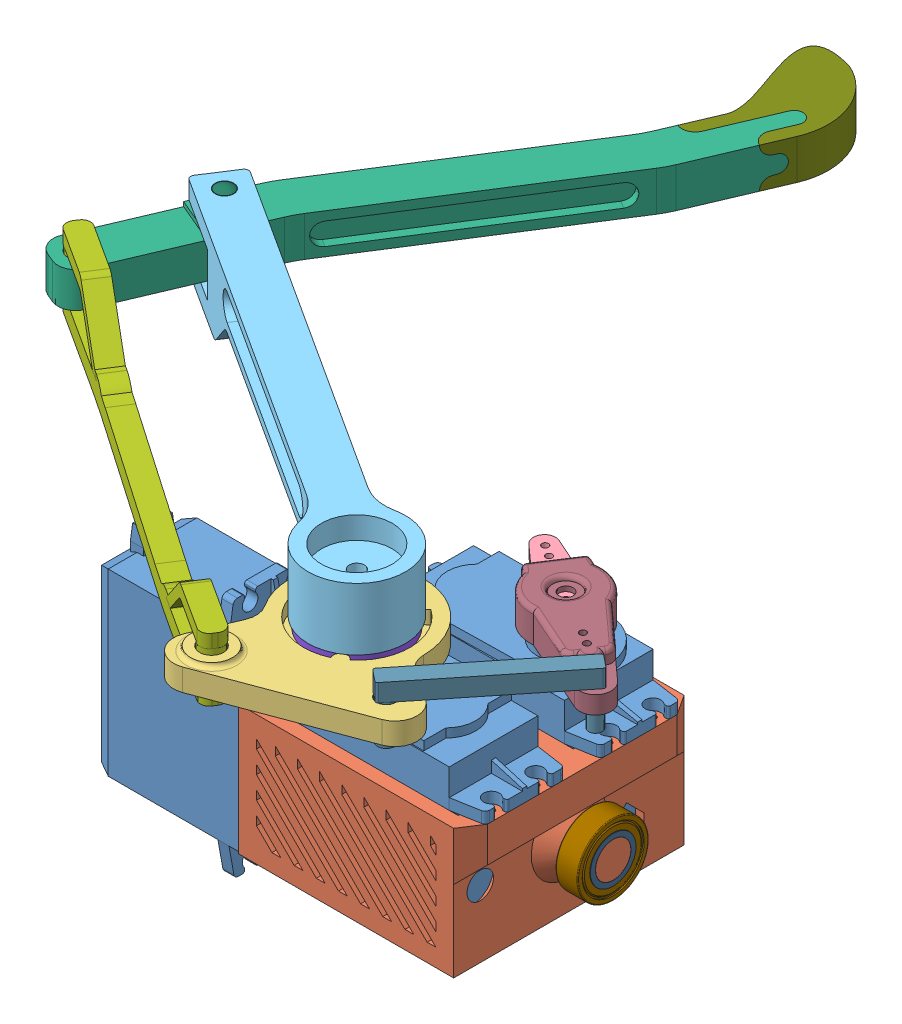
SolidWorks assembly Robot Assembly, configuration Default. Lengths in mm.
Overall size (181.61 84.3 186.42).
29 component instances, 16 part files, 41 mates.
Components (placement in the parent):
- MG996R-1: MG996R [Default] at (27.4949 -81.7725 169.9331) size (54.5 42.75 20)
- MG996R-2: MG996R [Default] at (27.4949 -81.7725 143.9331) x (-1 0 0) z (0 0 -1) size (54.5 42.75 20)
- MG996R-3: MG996R [Default] at (-44.8051 -79.1725 156.8317) x (0 -1 0) z (0 0 1) size (54.5 42.75 20)
- Servo Housing 2-1: Servo Housing 2 [Default] at (27.4949 -52.0225 169.9331) x (1 0 0) z (0 1 0) size (61.5 52 29.25)
- Rotating Piece-1: Rotating Piece [Default] at (16.9949 -42.0225 170.0344) x (-0.039952 0 -0.999202) z (0.999202 0 -0.039952) size (44.28 6 43.21)
- Double_Blade_Rudder-1: Double_Blade_Rudder [默认] at (37.9949 -36.7225 143.8317) x (0.544593 0 -0.8387) z (-0.8387 0 -0.544593) size (12.2 5.5 38)
- Upper Leg-1: Upper Leg [Default] at (-73.9237 -32.7225 117.2695) x (-0.542517 0 0.840045) z (0 1 0) size (22 116.4 18)
- Lower leg-1: Lower leg [Default] at (-14.4876 -27.2225 29.3622) x (0.92059 0 0.390531) z (0 -1 0) size (20.21 126 9.59)
- Long Connection Rod-1: Long Connection Rod [Default] at (10.6837 -42.0225 192.3035) x (0.542523 0 -0.840041) z (-0.840041 0 -0.542523) size (5 22 105.4)
- Circle Rudder-1: Circle Rudder [默认] at (0.2449 -68.6725 156.9331) x (0 0.962907 -0.269833) z (0 0.269833 0.962907) size (20.8 5.5 20.8)
- 688ZZ Bearing Assembly-2: 688ZZ Bearing Assembly [Default] at (59.2449 -68.6725 156.9331) x (0 -0.799794 -0.600275) z (1 0 0) size (17.99 17.98 5)
  - Outer Ring-1: Outer Ring [Default] at origin size (16 16 5)
  - Inner Ring-1: Inner Ring [Default] x (-0.241565 -0.970385 0) z (0 0 1) size (10.6 10.6 5)
  - Cage-1: Cage [Default] x (0.535517 0.844524 0) z (0 0 1) size (13.01 13.06 2.21)
  - 2mm Ball Bearing-1: 2mm Ball Bearing [Default] at (-5.0671 3.2131 0) x (0.050652 0.835774 0.546732) z (0.977207 -0.154478 0.145614) size (2 2 2)
  - 2mm Ball Bearing-2: 2mm Ball Bearing [Default] at (-5.988 -0.3789 0) x (-0.450278 0.705928 0.546732) z (0.881377 0.449412 0.145614) size (2 2 2)
  - 2mm Ball Bearing-3: 2mm Ball Bearing [Default] at (-4.6217 -3.8262 0) x (-0.779216 0.306441 0.546732) z (0.448891 0.881642 0.145614) size (2 2 2)
  - 2mm Ball Bearing-4: 2mm Ball Bearing [Default] at (-1.49 -5.812 0) x (-0.810521 -0.210096 0.546732) z (-0.155056 0.977115 0.145614) size (2 2 2)
  - 2mm Ball Bearing-5: 2mm Ball Bearing [Default] at (2.2108 -5.5778 0) x (-0.532234 -0.646383 0.546732) z (-0.699777 0.699363 0.145614) size (2 2 2)
  - 2mm Ball Bearing-6: 2mm Ball Bearing [Default] at (5.0671 -3.2131 0) x (-0.050652 -0.835774 0.546732) z (-0.977207 0.154478 0.145614) size (2 2 2)
  - 2mm Ball Bearing-7: 2mm Ball Bearing [Default] at (5.988 0.3789 0) x (0.450278 -0.705928 0.546732) z (-0.881377 -0.449412 0.145614) size (2 2 2)
  - 2mm Ball Bearing-8: 2mm Ball Bearing [Default] at (4.6217 3.8262 0) x (0.779216 -0.306441 0.546732) z (-0.448891 -0.881642 0.145614) size (2 2 2)
  - 2mm Ball Bearing-9: 2mm Ball Bearing [Default] at (1.49 5.812 0) x (0.810521 0.210096 0.546732) z (0.155056 -0.977115 0.145614) size (2 2 2)
  - 2mm Ball Bearing-10: 2mm Ball Bearing [Default] at (-2.2108 5.5778 0) x (0.532234 0.646383 0.546732) z (0.699777 -0.699363 0.145614) size (2 2 2)
- Circle Rudder-3: Circle Rudder [默认] at (16.9949 -36.7225 170.0344) x (-0.704797 0 -0.709409) z (-0.709409 0 0.704797) size (20.8 5.5 20.8)
- Servo Arm Mount-1: Servo Arm Mount [Default] at (37.9949 -36.7225 143.8317) x (-0.544593 0 0.8387) z (0 1 0) size (16.2 34.39 7.06)
- Short Connecting Rod-1: Short Connecting Rod [Default] at (59.4315 -36.7225 156.2089) x (-0.625381 0 0.780319) z (0 1 0) size (37.08 4 13)
- 91595A167_Dowel Pin-1: 91595A167_Dowel Pin [91595A167] at (-67.3495 -32.1225 115.5632) x (0.661086 0 -0.75031) z (0 -1 0) size (4 4 20)
- Foot-1: Foot [Default] at (-14.4876 -27.2225 29.3622) x (0.92059 0 0.390531) z (0 -1 0) size (22.97 31.5 9.59)
Mates (geometry in assembly coordinates):
- Coincident3: coincident aligned: plane of MG996R-1 through (16.9949 -44.0225 170.0344) normal (0 1 0); plane of MG996R-2 through (37.9949 -44.0225 143.8317) normal (0 1 0)
- Coincident4: coincident aligned: plane of MG996R-1 through (7.2449 -46.0225 179.9331) normal (-1 0 0); plane of MG996R-2 through (7.2449 -46.0225 133.9331) normal (-1 0 0)
- Distance1: distance = 6 mm anti-aligned: plane of MG996R-1 through (7.2449 -46.0225 159.9331) normal (0 0 -1); plane of MG996R-2 through (47.7449 -46.0225 153.9331) normal (0 0 1)
- Concentric1: concentric aligned: cylinder of MG996R-1 through (16.9949 -42.0225 170.0344) axis (0 1 0) radius 1.5; circle of Rotating Piece-1
- Coincident5: coincident anti-aligned: plane of MG996R-1 through (16.9949 -42.0225 170.0344) normal (0 1 0); plane of Rotating Piece-1 through (16.9949 -42.0225 170.0344) normal (0 -1 0)
- Coincident7: coincident anti-aligned: plane of MG996R-2 through (37.9949 -39.0225 143.8317) normal (0 1 0); plane of Double_Blade_Rudder-1 through (37.9949 -39.0225 143.8317) normal (0 -1 0)
- Concentric2: concentric aligned: cylinder of MG996R-2 through (37.9949 -42.0225 143.8317) axis (0 1 0) radius 1.5; cylinder of Double_Blade_Rudder-1 through (37.9949 -39.0225 143.8317) axis (0 1 0) radius 1.5
- Concentric3: concentric aligned: cylinder of Rotating Piece-1 through (16.9949 -40.0225 170.0344) axis (0 -1 0) radius 4.5; cylinder of Upper Leg-1 through (16.9949 -27.7225 170.0344) axis (0 -1 0) radius 1.7
- Concentric4: concentric aligned: cylinder of Upper Leg-1 through (-67.3495 -40.7225 115.5632) axis (0 1 0) radius 2.1; cylinder of Lower leg-1 through (-67.3495 -36.2225 115.5632) axis (0 1 0) radius 2
- Distance3: distance = 0.5 mm anti-aligned: plane of Lower leg-1 through (-14.4876 -27.2225 29.3622) normal (0 1 0); plane of Upper Leg-1 through (-65.2434 -26.7225 103.8288) normal (0 -1 0)
- LimitAngle3: limit planar angle = 1.561857 rad anti-aligned: plane of Lower leg-1 through (-22.5488 72.2991 167.5346) normal (-0.851754 0.472582 0.226234); plane of Upper Leg-1 through (-65.8745 -10.9193 112.7292) normal (0.165208 -0.889579 -0.425859)
- Coincident17: coincident anti-aligned: plane of Servo Housing 2-1 through (0.2449 -157.1001 169.9331) normal (-1 0 0); plane of Circle Rudder-1 through (0.2449 -68.6725 156.9331) normal (1 0 0)
- Concentric10: concentric aligned: circle of Servo Housing-1; circle of Circle Rudder-1
- Concentric11: concentric anti-aligned: cylinder of Servo Housing 2-1 through (61.7449 -68.6725 156.9331) axis (-1 0 0) radius 4; cylinder of 688ZZ Bearing Assembly-2/Inner Ring-1 through (66.0003 -68.6725 156.9331) axis (1 0 0) radius 4
- Coincident18: coincident aligned: plane of Servo Housing 2-1 through (61.7449 -52.0225 169.9331) normal (1 0 0); plane of 688ZZ Bearing Assembly-2/Inner Ring-1 through (61.7449 -73.4162 154.9282) normal (1 0 0)
- Coincident19: coincident anti-aligned: plane of MG996R-1 through (16.9949 -39.0225 170.0344) normal (0 1 0); plane of Circle Rudder-3 through (16.9949 -39.0225 170.0344) normal (0 -1 0)
- Concentric12: concentric aligned: cylinder of MG996R-1 through (16.9949 -42.0225 170.0344) axis (0 1 0) radius 1.5; cylinder of Circle Rudder-3 through (16.9949 -39.0225 170.0344) axis (0 1 0) radius 1.5
- Coincident20: coincident anti-aligned: plane of Upper Leg-1 through (16.9949 -36.7225 170.0344) normal (0 -1 0); plane of Circle Rudder-3 through (16.9949 -36.7225 170.0344) normal (0 1 0)
- InPlace2: in place: plane of ? through (-72.3336 35.5583 10.554) normal (0 1 0); plane of ? through (0 35.5583 0) normal (0 1 0); moOrthogonalPlaneRef_w of ? through (-72.3336 35.5583 10.554) normal (0 1 0); plane of ? through (0 35.5583 0) normal (0 0 -1); plane of ? through (-72.3336 35.5583 10.554) normal (0 1 0); plane of ? through (0 35.5583 0) normal (1 0 0); plane of Double_Blade_Rudder-1 through (37.9949 -36.7225 143.8317) normal (0 1 0); unknown of Servo Arm Mount-1
- Coincident21: coincident aligned: plane of Double_Blade_Rudder-1; plane of Servo Arm Mount-1
- Coincident22: coincident aligned: moOrthogonalPlaneRef_w of Double_Blade_Rudder-1; plane of Servo Arm Mount-1 through (37.9949 -36.7225 143.8317) normal (0.8387 0 0.544593)
- Coincident23: coincident anti-aligned: moOrthogonalPlaneRef_w of Double_Blade_Rudder-1; plane of Servo Arm Mount-1 through (37.9949 -36.7225 143.8317) normal (-0.544593 0 0.8387)
- Concentric15: concentric anti-aligned: cylinder of Rotating Piece-1 through (35.9325 -37.0225 182.3318) axis (0 -1 0) radius 2.2; cylinder of Short Connecting Rod-1 through (35.9325 -45.7225 182.3318) axis (0 1 0) radius 2
- Concentric16: concentric aligned: cylinder of Short Connecting Rod-1 through (56.9328 -45.7225 156.1286) axis (0 1 0) radius 1.5; cylinder of Servo Arm Mount-1 through (56.9328 -40.7225 156.1286) axis (0 1 0) radius 1.7
- Concentric17: concentric aligned: cylinder of Double_Blade_Rudder-1 through (37.9949 -39.0225 143.8317) axis (0 1 0) radius 1.5; cylinder of Servo Arm Mount-1 through (37.9949 -36.8225 143.8317) axis (0 1 0) radius 1.6
- Concentric18: concentric anti-aligned: cylinder of Upper Leg-1 through (-67.3495 -40.7225 115.5632) axis (0 1 0) radius 2.1; cylinder of 91595A167_Dowel Pin-1 through (-67.3495 -42.1225 115.5632) axis (0 -1 0) radius 2
- Coincident32: coincident anti-aligned: plane of Upper Leg-1 through (-73.9237 -22.7225 117.2695) normal (0 1 0); circle of 91595A167_Dowel Pin-1
- Concentric24: concentric aligned: cylinder of Circle Rudder-1 through (-5.2551 -68.6725 156.9331) axis (1 0 0) radius 3; cylinder of MG996R-3 through (-5.0551 -68.6725 156.9331) axis (1 0 0) radius 1.5
- Concentric26: concentric aligned: cylinder of Rotating Piece-1 through (7.2273 -37.0225 193.0473) axis (0 -1 0) radius 2.7; cylinder of Long Connection Rod-1 through (7.2273 -34.8225 193.0473) axis (0 -1 0) radius 2.5
- Concentric27: concentric anti-aligned: cylinder of Lower leg-1 through (-77.1128 -36.2225 138.5779) axis (0 1 0) radius 2.6; cylinder of Long Connection Rod-1 through (-77.1128 -27.0225 138.5779) axis (0 -1 0) radius 2.5
- Concentric28: concentric anti-aligned: cylinder of Lower leg-1 through (-77.1128 -36.2225 138.5779) axis (0 1 0) radius 2.6; cylinder of Long Connection Rod-1 through (-77.1128 -27.0225 138.5779) axis (0 -1 0) radius 2.5
- Coincident34: coincident anti-aligned: plane of Rotating Piece-1 through (16.9949 -42.0225 170.0344) normal (0 -1 0); plane of Long Connection Rod-1 through (10.6837 -42.0225 192.3035) normal (0 1 0)
- Coincident37: coincident anti-aligned: plane of Servo Arm Mount-1 through (37.9949 -36.7225 143.8317) normal (0 1 0); plane of Short Connecting Rod-1 through (59.4315 -36.7225 156.2089) normal (0 -1 0)
- LimitDistance1: limit distance = 0 mm anti-aligned: plane of Circle Rudder-1 through (-2.0551 -68.6725 156.9331) normal (-1 0 0); plane of MG996R-3 through (-2.0551 -68.6725 156.9331) normal (1 0 0)
- Tangent6: tangent aligned: cylinder of Lower leg-1 through (-21.4337 -27.2225 32.9331) axis (0 -1 0) radius 2
- Tangent7: tangent: circle of assembly; circle of Lower leg-1; plane of assembly
- Parallel1: parallel anti-aligned: unknown of Servo Housing 2-1
- Parallel2: parallel anti-aligned: plane of MG996R-3 through (-9.0551 -58.9225 146.8317) normal (0 0 -1)
- Concentric29: concentric aligned: cylinder of Lower leg-1 through (-27.4869 -31.7225 47.2022) axis (-0.92059 0 -0.390531) radius 2; cylinder of Foot-1 through (-27.4869 -31.7225 47.2022) axis (-0.92059 0 -0.390531) radius 2
- Coincident38: coincident anti-aligned: plane of Lower leg-1 through (-23.2749 -27.2225 32.152) normal (-0.92059 0 -0.390531); plane of Foot-1 through (-23.2749 -27.2225 32.152) normal (0.92059 0 0.390531)
- Coincident39: coincident aligned: plane of Lower leg-1 through (-14.4876 -27.2225 29.3622) normal (0 1 0); plane of Foot-1 through (-14.4876 -27.2225 29.3622) normal (0 1 0)
